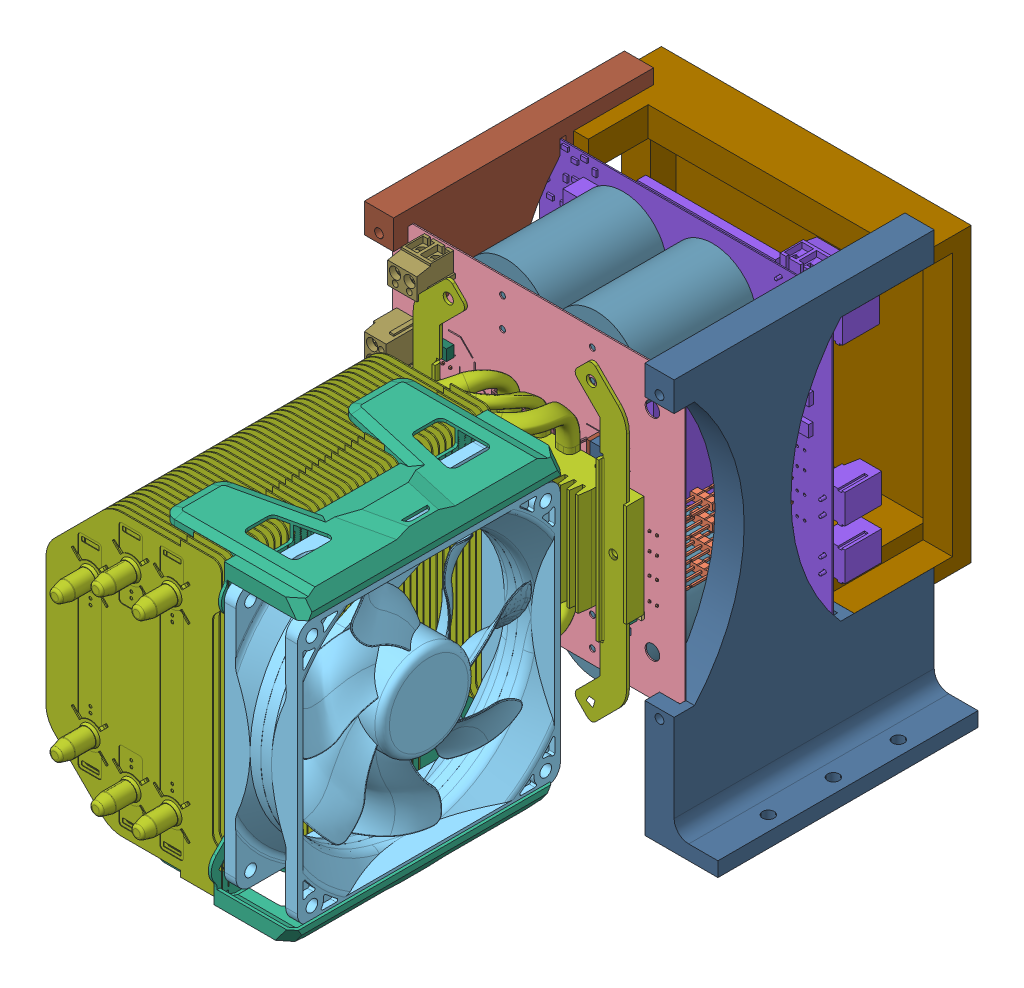
SolidWorks assembly conversor, configuration Default. Lengths in mm.
Overall size (196.64 140 240.72).
331 component instances, 30 part files, 12 mates.
Components (placement in the parent):
- inversor_rev2-1: inversor_rev2 [Default] at (-42.011 -49.0953 13.8297) size (100.07 109.25 61.05)
  - inversor_rev2.step-1: inversor_rev2.step [Default] at origin size (100.07 109.25 61.05)
    - R11.step-1: R11.step [Default] at origin size (1.4 2.15 0.65)
      - 1052595968.step-1: 1052595968.step [Default] at (72.136 29.972 0) size (1.4 2.15 0.65)
        - Extruded.step-1: Extruded.step [Default] at origin size (1.4 2.15 0.65)
    - R10.step-1: R10.step [Default] at origin size (1.4 2.15 0.65)
      - 1052595968.step-1: 1052595968.step [Default] at (74.93 29.972 0) size (1.4 2.15 0.65)
        - Extruded.step-1: Extruded.step [Default] at origin size (1.4 2.15 0.65)
    - P8.step-1: P8.step [Default] at origin size (7.72 2.67 47.1)
      - zl201-3_p2-54_l7-62_w2-54_h8-89.step-1: zl201-3_p2-54_l7-62_w2-54_h8-89.step [Default] at (83.5661 26.6699 -43.4013) x (1 0 0) z (0 -1 0) size (7.62 11.94 2.54)
      - zl201-3_p2-54_l7-62_w2-54_h8-89.step-2: zl201-3_p2-54_l7-62_w2-54_h8-89.step [Default] at (83.6675 26.7717 -20) x (1 0 0) z (0 -1 0) size (7.62 11.94 2.54)
      - zl201-3_p2-54_l7-62_w2-54_h8-89.step-3: zl201-3_p2-54_l7-62_w2-54_h8-89.step [Default] at (83.6675 26.7717 -2.4013) x (1 0 0) z (0 1 0) size (7.62 11.94 2.54)
      - zl201-3_p2-54_l7-62_w2-54_h8-89.step-4: zl201-3_p2-54_l7-62_w2-54_h8-89.step [Default] at (83.6675 26.7971 -31.9013) x (1 0 0) z (0 -1 0) size (7.62 11.94 2.54)
    - C19.step-1: C19.step [Default] at origin size (1.45 2.2 1.1)
      - 1052595832.step-1: 1052595832.step [Default] at (83.566 21.59 0) size (1.45 2.2 1.1)
        - Extruded-4.step-1: Extruded-4.step [Default] at origin size (1.45 2.2 1.1)
    - C18.step-1: C18.step [Default] at origin size (1.45 2.2 1.1)
      - 1052595832.step-1: 1052595832.step [Default] at (69.342 30.353 0) size (1.45 2.2 1.1)
        - Extruded-4.step-1: Extruded-4.step [Default] at origin size (1.45 2.2 1.1)
    - C11.step-1: C11.step [Default] at origin size (3.4 1.8 1.35)
      - 1052596240.step-1: 1052596240.step [Default] at (79.502 24.892 -1.7513) size (3.4 1.8 1.35)
        - Extruded-1.step-1: Extruded-1.step [Default] at origin size (3.4 1.8 1.35)
    - C10.step-1: C10.step [Default] at origin size (4.3 7.5 4)
      - 1052596648.step-1: 1052596648.step [Default] at (79.502 22.352 0) size (4.3 4.9 4)
        - Extruded-2.step-1: Extruded-2.step [Default] at origin size (4.3 4.9 4)
      - 1052596784.step-1: 1052596784.step [Default] at (79.502 19.252 0) size (4.3 1.3 4)
        - Extruded-3.step-1: Extruded-3.step [Default] at origin size (4.3 1.3 4)
      - 1052596784.step-2: 1052596784.step [Default] at (79.502 25.452 0) size (4.3 1.3 4)
        - Extruded-3.step-1: Extruded-3.step [Default] at origin size (4.3 1.3 4)
    - C22.step-1: C22.step [Default] at origin size (1.45 2.2 1.1)
      - 1052597056.step-1: 1052597056.step [Default] at (74.93 32.512 -1.7513) size (1.45 2.2 1.1)
        - Extruded-4.step-1: Extruded-4.step [Default] at origin size (1.45 2.2 1.1)
    - C21.step-1: C21.step [Default] at origin size (4.3 7.5 4)
      - 1052596648.step-1: 1052596648.step [Default] at (79.502 31.242 0) size (4.3 4.9 4)
        - Extruded-2.step-1: Extruded-2.step [Default] at origin size (4.3 4.9 4)
      - 1052596784.step-1: 1052596784.step [Default] at (79.502 28.142 0) size (4.3 1.3 4)
        - Extruded-3.step-1: Extruded-3.step [Default] at origin size (4.3 1.3 4)
      - 1052596784.step-2: 1052596784.step [Default] at (79.502 34.342 0) size (4.3 1.3 4)
        - Extruded-3.step-1: Extruded-3.step [Default] at origin size (4.3 1.3 4)
    - C20.step-1: C20.step [Default] at origin size (4.3 7.5 4)
      - 1052596648.step-1: 1052596648.step [Default] at (79.248 31.242 -4.4013) size (4.3 4.9 4)
        - Extruded-2.step-1: Extruded-2.step [Default] at origin size (4.3 4.9 4)
      - 1052596784.step-1: 1052596784.step [Default] at (79.248 28.142 -4.4013) size (4.3 1.3 4)
        - Extruded-3.step-1: Extruded-3.step [Default] at origin size (4.3 1.3 4)
      - 1052596784.step-2: 1052596784.step [Default] at (79.248 34.342 -4.4013) size (4.3 1.3 4)
        - Extruded-3.step-1: Extruded-3.step [Default] at origin size (4.3 1.3 4)
    - D3.step-1: D3.step [Default] at origin size (20 1.52 1.52)
      - do35_d1-5_l3.step-1: do35_d1-5_l3.step [Default] at (49.9079 33.2429 -1.4013) x (1 0 0) z (0 0 -1) size (20 1.52 1.52)
        - Open CASCADE STEP translator 6.8 1.12.1.1.step-1: Open CASCADE STEP translator 6.8 1.12.1.1.step [Default] at origin size (20 1.52 1.52)
        - Open CASCADE STEP translator 6.8 1.12.1.2.step-1: Open CASCADE STEP translator 6.8 1.12.1.2.step [Default] at origin
    - D2.step-1: D2.step [Default] at origin size (20 1.52 1.52)
      - do35_d1-5_l3.step-1: do35_d1-5_l3.step [Default] at (49.9619 38.0745 -1.4013) x (1 0 0) z (0 0 -1) size (20 1.52 1.52)
        - Open CASCADE STEP translator 6.8 1.12.1.1.step-1: Open CASCADE STEP translator 6.8 1.12.1.1.step [Default] at origin size (20 1.52 1.52)
        - Open CASCADE STEP translator 6.8 1.12.1.2.step-1: Open CASCADE STEP translator 6.8 1.12.1.2.step [Default] at origin
    - D1.step-1: D1.step [Default] at origin size (20 1.52 1.52)
      - do35_d1-5_l3.step-1: do35_d1-5_l3.step [Default] at (49.9959 42.6465 -1.4013) x (1 0 0) z (0 0 -1) size (20 1.52 1.52)
        - Open CASCADE STEP translator 6.8 1.12.1.1.step-1: Open CASCADE STEP translator 6.8 1.12.1.1.step [Default] at origin size (20 1.52 1.52)
        - Open CASCADE STEP translator 6.8 1.12.1.2.step-1: Open CASCADE STEP translator 6.8 1.12.1.2.step [Default] at origin
    - R13.step-1: R13.step [Default] at origin size (2.15 1.4 0.65)
      - 1052596104.step-1: 1052596104.step [Default] at (58.928 35.56 -1.0513) size (2.15 1.4 0.65)
        - Extruded-5.step-1: Extruded-5.step [Default] at origin size (2.15 1.4 0.65)
    - R15.step-1: R15.step [Default] at origin size (2.15 1.4 0.65)
      - 1052596104.step-1: 1052596104.step [Default] at (40.132 33.782 -1.0513) size (2.15 1.4 0.65)
        - Extruded-5.step-1: Extruded-5.step [Default] at origin size (2.15 1.4 0.65)
    - R14.step-1: R14.step [Default] at origin size (2.15 1.4 0.65)
      - 1052596104.step-1: 1052596104.step [Default] at (40.386 38.608 -1.0513) size (2.15 1.4 0.65)
        - Extruded-5.step-1: Extruded-5.step [Default] at origin size (2.15 1.4 0.65)
    - R12.step-1: R12.step [Default] at origin size (2.15 1.4 0.65)
      - 1052596104.step-1: 1052596104.step [Default] at (40.386 43.434 -1.0513) size (2.15 1.4 0.65)
        - Extruded-5.step-1: Extruded-5.step [Default] at origin size (2.15 1.4 0.65)
    - C26.step-1: C26.step [Default] at origin size (2.2 1.45 1.1)
      - 1052596920.step-1: 1052596920.step [Default] at (41.402 40.64 -1.5013) size (2.2 1.45 1.1)
        - Extruded-6.step-1: Extruded-6.step [Default] at origin size (2.2 1.45 1.1)
    - C25.step-1: C25.step [Default] at origin size (2.2 1.45 1.1)
      - 1052596920.step-1: 1052596920.step [Default] at (41.402 35.814 -1.5013) size (2.2 1.45 1.1)
        - Extruded-6.step-1: Extruded-6.step [Default] at origin size (2.2 1.45 1.1)
    - C24.step-1: C24.step [Default] at origin size (2.2 1.45 1.1)
      - 1052596920.step-1: 1052596920.step [Default] at (41.402 30.988 -1.5013) size (2.2 1.45 1.1)
        - Extruded-6.step-1: Extruded-6.step [Default] at origin size (2.2 1.45 1.1)
    - R17.step-1: R17.step [Default] at origin size (1.4 2.15 0.65)
      - 1052595968.step-1: 1052595968.step [Default] at (78.994 14.478 0) size (1.4 2.15 0.65)
        - Extruded.step-1: Extruded.step [Default] at origin size (1.4 2.15 0.65)
    - P1.step-1: P1.step [Default] at origin size (7.72 2.67 47.1)
      - zl201-3_p2-54_l7-62_w2-54_h8-89.step-1: zl201-3_p2-54_l7-62_w2-54_h8-89.step [Default] at (83.5661 34.2899 -43.4013) x (1 0 0) z (0 -1 0) size (7.62 11.94 2.54)
      - zl201-3_p2-54_l7-62_w2-54_h8-89.step-2: zl201-3_p2-54_l7-62_w2-54_h8-89.step [Default] at (83.6675 34.3917 -20) x (1 0 0) z (0 -1 0) size (7.62 11.94 2.54)
      - zl201-3_p2-54_l7-62_w2-54_h8-89.step-3: zl201-3_p2-54_l7-62_w2-54_h8-89.step [Default] at (83.6675 34.3917 -2.4013) x (1 0 0) z (0 1 0) size (7.62 11.94 2.54)
      - zl201-3_p2-54_l7-62_w2-54_h8-89.step-4: zl201-3_p2-54_l7-62_w2-54_h8-89.step [Default] at (83.6675 34.4171 -31.9013) x (1 0 0) z (0 -1 0) size (7.62 11.94 2.54)
    - C17.step-1: C17.step [Default] at origin size (2.2 1.45 1.1)
      - 1052596920.step-1: 1052596920.step [Default] at (75.946 47.498 -1.5013) size (2.2 1.45 1.1)
        - Extruded-6.step-1: Extruded-6.step [Default] at origin size (2.2 1.45 1.1)
    - C16.step-1: C16.step [Default] at origin size (2.2 1.45 1.1)
      - 1052596920.step-1: 1052596920.step [Default] at (75.946 41.402 -1.5013) size (2.2 1.45 1.1)
        - Extruded-6.step-1: Extruded-6.step [Default] at origin size (2.2 1.45 1.1)
    - C15.step-1: C15.step [Default] at origin size (2.2 1.45 1.1)
      - 1052596920.step-1: 1052596920.step [Default] at (75.946 45.466 -1.5013) size (2.2 1.45 1.1)
        - Extruded-6.step-1: Extruded-6.step [Default] at origin size (2.2 1.45 1.1)
    - C14.step-1: C14.step [Default] at origin size (2.2 1.45 1.1)
      - 1052596920.step-1: 1052596920.step [Default] at (75.946 39.37 -1.5013) size (2.2 1.45 1.1)
        - Extruded-6.step-1: Extruded-6.step [Default] at origin size (2.2 1.45 1.1)
    - C13.step-1: C13.step [Default] at origin size (2.2 1.45 1.1)
      - 1052596920.step-1: 1052596920.step [Default] at (75.946 43.434 -1.5013) size (2.2 1.45 1.1)
        - Extruded-6.step-1: Extruded-6.step [Default] at origin size (2.2 1.45 1.1)
    - C12.step-1: C12.step [Default] at origin size (2.2 1.45 1.1)
      - 1052596920.step-1: 1052596920.step [Default] at (75.946 37.338 -1.5013) size (2.2 1.45 1.1)
        - Extruded-6.step-1: Extruded-6.step [Default] at origin size (2.2 1.45 1.1)
    - P2.step-1: P2.step [Default] at origin size (7.72 2.67 47.1)
      - zl201-3_p2-54_l7-62_w2-54_h8-89.step-1: zl201-3_p2-54_l7-62_w2-54_h8-89.step [Default] at (83.5661 47.4979 -43.4013) x (1 0 0) z (0 -1 0) size (7.62 11.94 2.54)
      - zl201-3_p2-54_l7-62_w2-54_h8-89.step-2: zl201-3_p2-54_l7-62_w2-54_h8-89.step [Default] at (83.6675 47.5997 -20) x (1 0 0) z (0 -1 0) size (7.62 11.94 2.54)
      - zl201-3_p2-54_l7-62_w2-54_h8-89.step-3: zl201-3_p2-54_l7-62_w2-54_h8-89.step [Default] at (83.6675 47.5997 -2.4013) x (1 0 0) z (0 1 0) size (7.62 11.94 2.54)
      - zl201-3_p2-54_l7-62_w2-54_h8-89.step-4: zl201-3_p2-54_l7-62_w2-54_h8-89.step [Default] at (83.6675 47.6251 -31.9013) x (1 0 0) z (0 -1 0) size (7.62 11.94 2.54)
    - P3.step-1: P3.step [Default] at origin size (7.72 2.67 47.1)
      - zl201-3_p2-54_l7-62_w2-54_h8-89.step-1: zl201-3_p2-54_l7-62_w2-54_h8-89.step [Default] at (83.5661 41.5289 -43.4013) x (1 0 0) z (0 -1 0) size (7.62 11.94 2.54)
      - zl201-3_p2-54_l7-62_w2-54_h8-89.step-2: zl201-3_p2-54_l7-62_w2-54_h8-89.step [Default] at (83.6675 41.6307 -20) x (1 0 0) z (0 -1 0) size (7.62 11.94 2.54)
      - zl201-3_p2-54_l7-62_w2-54_h8-89.step-3: zl201-3_p2-54_l7-62_w2-54_h8-89.step [Default] at (83.6675 41.6307 -2.4013) x (1 0 0) z (0 1 0) size (7.62 11.94 2.54)
      - zl201-3_p2-54_l7-62_w2-54_h8-89.step-4: zl201-3_p2-54_l7-62_w2-54_h8-89.step [Default] at (83.6675 41.6561 -31.9013) x (1 0 0) z (0 -1 0) size (7.62 11.94 2.54)
    - R6.step-1: R6.step [Default] at origin size (2.15 1.4 0.65)
      - 1052596104.step-1: 1052596104.step [Default] at (75.946 37.338 0) size (2.15 1.4 0.65)
        - Extruded-5.step-1: Extruded-5.step [Default] at origin size (2.15 1.4 0.65)
    - R5.step-1: R5.step [Default] at origin size (2.15 1.4 0.65)
      - 1052596104.step-1: 1052596104.step [Default] at (75.946 39.37 0) size (2.15 1.4 0.65)
        - Extruded-5.step-1: Extruded-5.step [Default] at origin size (2.15 1.4 0.65)
    - R4.step-1: R4.step [Default] at origin size (2.15 1.4 0.65)
      - 1052596104.step-1: 1052596104.step [Default] at (75.946 41.402 0) size (2.15 1.4 0.65)
        - Extruded-5.step-1: Extruded-5.step [Default] at origin size (2.15 1.4 0.65)
    - R3.step-1: R3.step [Default] at origin size (2.15 1.4 0.65)
      - 1052596104.step-1: 1052596104.step [Default] at (75.946 43.434 0) size (2.15 1.4 0.65)
        - Extruded-5.step-1: Extruded-5.step [Default] at origin size (2.15 1.4 0.65)
    - R2.step-1: R2.step [Default] at origin size (2.15 1.4 0.65)
      - 1052596104.step-1: 1052596104.step [Default] at (75.946 45.466 0) size (2.15 1.4 0.65)
        - Extruded-5.step-1: Extruded-5.step [Default] at origin size (2.15 1.4 0.65)
    - R1.step-1: R1.step [Default] at origin size (2.15 1.4 0.65)
      - 1052596104.step-1: 1052596104.step [Default] at (75.946 47.498 0) size (2.15 1.4 0.65)
        - Extruded-5.step-1: Extruded-5.step [Default] at origin size (2.15 1.4 0.65)
    - C8.step-1: C8.step [Default] at origin size (7.5 4.3 4)
      - 1052596376.step-1: 1052596376.step [Default] at (75.211 51.816 0) size (4.9 4.3 4)
        - Extruded-7.step-1: Extruded-7.step [Default] at origin size (4.9 4.3 4)
      - 1052596512.step-1: 1052596512.step [Default] at (72.111 51.816 0) size (1.3 4.3 4)
        - Extruded-8.step-1: Extruded-8.step [Default] at origin size (1.3 4.3 4)
      - 1052596512.step-2: 1052596512.step [Default] at (78.311 51.816 0) size (1.3 4.3 4)
        - Extruded-8.step-1: Extruded-8.step [Default] at origin size (1.3 4.3 4)
    - C6.step-1: C6.step [Default] at origin size (7.5 4.3 4)
      - 1052596376.step-1: 1052596376.step [Default] at (71.855 58.928 0) size (4.9 4.3 4)
        - Extruded-7.step-1: Extruded-7.step [Default] at origin size (4.9 4.3 4)
      - 1052596512.step-1: 1052596512.step [Default] at (74.955 58.928 0) size (1.3 4.3 4)
        - Extruded-8.step-1: Extruded-8.step [Default] at origin size (1.3 4.3 4)
      - 1052596512.step-2: 1052596512.step [Default] at (68.755 58.928 0) size (1.3 4.3 4)
        - Extruded-8.step-1: Extruded-8.step [Default] at origin size (1.3 4.3 4)
    - C4.step-1: C4.step [Default] at origin size (7.5 4.3 4)
      - 1052596376.step-1: 1052596376.step [Default] at (72.136 65.786 0) size (4.9 4.3 4)
        - Extruded-7.step-1: Extruded-7.step [Default] at origin size (4.9 4.3 4)
      - 1052596512.step-1: 1052596512.step [Default] at (75.236 65.786 0) size (1.3 4.3 4)
        - Extruded-8.step-1: Extruded-8.step [Default] at origin size (1.3 4.3 4)
      - 1052596512.step-2: 1052596512.step [Default] at (69.036 65.786 0) size (1.3 4.3 4)
        - Extruded-8.step-1: Extruded-8.step [Default] at origin size (1.3 4.3 4)
    - -VDC1.step-1: -VDC1.step [Default] at origin size (10.6 9 17)
      - SCREW_TERMINAL_BLOCK_5MM.step-1: SCREW_TERMINAL_BLOCK_5MM.step [Default] at (20.1591 6.4347 2) x (-1 0 0) z (0 1 0) size (10.6 17 9)
    - +VDC1.step-1: +VDC1.step [Default] at origin size (10.6 9 17)
      - SCREW_TERMINAL_BLOCK_5MM.step-1: SCREW_TERMINAL_BLOCK_5MM.step [Default] at (10.9959 90.0853 2) x (1 0 0) z (0 -1 0) size (10.6 17 9)
    - P7.step-1: P7.step [Default] at origin size (7.72 2.67 47.1)
      - zl201-3_p2-54_l7-62_w2-54_h8-89.step-1: zl201-3_p2-54_l7-62_w2-54_h8-89.step [Default] at (18.0339 26.1621 -43.4013) x (-1 0 0) z (0 1 0) size (7.62 11.94 2.54)
      - zl201-3_p2-54_l7-62_w2-54_h8-89.step-2: zl201-3_p2-54_l7-62_w2-54_h8-89.step [Default] at (17.9325 26.0603 -20) x (-1 0 0) z (0 1 0) size (7.62 11.94 2.54)
      - zl201-3_p2-54_l7-62_w2-54_h8-89.step-3: zl201-3_p2-54_l7-62_w2-54_h8-89.step [Default] at (17.9325 26.0603 -2.4013) x (-1 0 0) z (0 -1 0) size (7.62 11.94 2.54)
      - zl201-3_p2-54_l7-62_w2-54_h8-89.step-4: zl201-3_p2-54_l7-62_w2-54_h8-89.step [Default] at (17.9325 26.0349 -31.9013) x (-1 0 0) z (0 1 0) size (7.62 11.94 2.54)
    - P6.step-1: P6.step [Default] at origin size (7.72 2.67 47.1)
      - zl201-3_p2-54_l7-62_w2-54_h8-89.step-1: zl201-3_p2-54_l7-62_w2-54_h8-89.step [Default] at (18.0339 35.8141 -43.4013) x (-1 0 0) z (0 1 0) size (7.62 11.94 2.54)
      - zl201-3_p2-54_l7-62_w2-54_h8-89.step-2: zl201-3_p2-54_l7-62_w2-54_h8-89.step [Default] at (17.9325 35.7123 -20) x (-1 0 0) z (0 1 0) size (7.62 11.94 2.54)
      - zl201-3_p2-54_l7-62_w2-54_h8-89.step-3: zl201-3_p2-54_l7-62_w2-54_h8-89.step [Default] at (17.9325 35.7123 -2.4013) x (-1 0 0) z (0 -1 0) size (7.62 11.94 2.54)
      - zl201-3_p2-54_l7-62_w2-54_h8-89.step-4: zl201-3_p2-54_l7-62_w2-54_h8-89.step [Default] at (17.9325 35.6869 -31.9013) x (-1 0 0) z (0 1 0) size (7.62 11.94 2.54)
    - P5.step-1: P5.step [Default] at origin size (7.72 2.67 47.1)
      - zl201-3_p2-54_l7-62_w2-54_h8-89.step-1: zl201-3_p2-54_l7-62_w2-54_h8-89.step [Default] at (18.0339 50.0381 -43.4013) x (-1 0 0) z (0 1 0) size (7.62 11.94 2.54)
      - zl201-3_p2-54_l7-62_w2-54_h8-89.step-2: zl201-3_p2-54_l7-62_w2-54_h8-89.step [Default] at (17.9325 49.9363 -20) x (-1 0 0) z (0 1 0) size (7.62 11.94 2.54)
      - zl201-3_p2-54_l7-62_w2-54_h8-89.step-3: zl201-3_p2-54_l7-62_w2-54_h8-89.step [Default] at (17.9325 49.9363 -2.4013) x (-1 0 0) z (0 -1 0) size (7.62 11.94 2.54)
      - zl201-3_p2-54_l7-62_w2-54_h8-89.step-4: zl201-3_p2-54_l7-62_w2-54_h8-89.step [Default] at (17.9325 49.9109 -31.9013) x (-1 0 0) z (0 1 0) size (7.62 11.94 2.54)
    - P4.step-1: P4.step [Default] at origin size (7.72 2.67 47.1)
      - zl201-3_p2-54_l7-62_w2-54_h8-89.step-1: zl201-3_p2-54_l7-62_w2-54_h8-89.step [Default] at (18.0339 61.9761 -43.4013) x (-1 0 0) z (0 1 0) size (7.62 11.94 2.54)
      - zl201-3_p2-54_l7-62_w2-54_h8-89.step-2: zl201-3_p2-54_l7-62_w2-54_h8-89.step [Default] at (17.9325 61.8743 -20) x (-1 0 0) z (0 1 0) size (7.62 11.94 2.54)
      - zl201-3_p2-54_l7-62_w2-54_h8-89.step-3: zl201-3_p2-54_l7-62_w2-54_h8-89.step [Default] at (17.9325 61.8743 -2.4013) x (-1 0 0) z (0 -1 0) size (7.62 11.94 2.54)
      - zl201-3_p2-54_l7-62_w2-54_h8-89.step-4: zl201-3_p2-54_l7-62_w2-54_h8-89.step [Default] at (17.9325 61.8489 -31.9013) x (-1 0 0) z (0 1 0) size (7.62 11.94 2.54)
    - W1.step-1: W1.step [Default] at origin size (9 10.6 17)
      - SCREW_TERMINAL_BLOCK_5MM.step-1: SCREW_TERMINAL_BLOCK_5MM.step [Default] at (10.4987 39.4909 2) x (0 1 0) z (1 0 0) size (10.6 17 9)
    - V1.step-1: V1.step [Default] at origin size (9 10.6 17)
      - SCREW_TERMINAL_BLOCK_5MM.step-1: SCREW_TERMINAL_BLOCK_5MM.step [Default] at (10.4987 50.9209 2) x (0 1 0) z (1 0 0) size (10.6 17 9)
    - U1.step-1: U1.step [Default] at origin size (9 10.6 17)
      - SCREW_TERMINAL_BLOCK_5MM.step-1: SCREW_TERMINAL_BLOCK_5MM.step [Default] at (10.4987 62.3509 2) x (0 1 0) z (1 0 0) size (10.6 17 9)
    - C3.step-1: C3.step [Default] at origin size (3.4 1.8 1.35)
      - 1052596240.step-1: 1052596240.step [Default] at (16.51 52.578 -1.7513) size (3.4 1.8 1.35)
        - Extruded-1.step-1: Extruded-1.step [Default] at origin size (3.4 1.8 1.35)
    - C2.step-1: C2.step [Default] at origin size (3.4 1.8 1.35)
      - 1052596240.step-1: 1052596240.step [Default] at (16.637 64.516 -1.7513) size (3.4 1.8 1.35)
        - Extruded-1.step-1: Extruded-1.step [Default] at origin size (3.4 1.8 1.35)
    - C1.step-1: C1.step [Default] at origin size (3.4 1.8 1.35)
      - 1052596240.step-1: 1052596240.step [Default] at (16.51 38.354 -1.7513) size (3.4 1.8 1.35)
        - Extruded-1.step-1: Extruded-1.step [Default] at origin size (3.4 1.8 1.35)
    - U2.step-1: U2.step [Default] at origin size (29.83 36.3 7.7)
      - User_Library-Cipos-mini-PCB.step-1: User_Library-Cipos-mini-PCB.step [Default] at (38.058 67.0707 2.5987) x (0 1 0) z (1 0 0) size (36.3 7.7 29.83)
    - C7.step-1: C7.step [Default] at origin size (7.5 4.3 4)
      - 1052596376.step-1: 1052596376.step [Default] at (72.136 58.928 -4.4013) size (4.9 4.3 4)
        - Extruded-7.step-1: Extruded-7.step [Default] at origin size (4.9 4.3 4)
      - 1052596512.step-1: 1052596512.step [Default] at (75.236 58.928 -4.4013) size (1.3 4.3 4)
        - Extruded-8.step-1: Extruded-8.step [Default] at origin size (1.3 4.3 4)
      - 1052596512.step-2: 1052596512.step [Default] at (69.036 58.928 -4.4013) size (1.3 4.3 4)
        - Extruded-8.step-1: Extruded-8.step [Default] at origin size (1.3 4.3 4)
    - C5.step-1: C5.step [Default] at origin size (7.5 4.3 4)
      - 1052596376.step-1: 1052596376.step [Default] at (71.882 65.786 -4.4013) size (4.9 4.3 4)
        - Extruded-7.step-1: Extruded-7.step [Default] at origin size (4.9 4.3 4)
      - 1052596512.step-1: 1052596512.step [Default] at (74.982 65.786 -4.4013) size (1.3 4.3 4)
        - Extruded-8.step-1: Extruded-8.step [Default] at origin size (1.3 4.3 4)
      - 1052596512.step-2: 1052596512.step [Default] at (68.782 65.786 -4.4013) size (1.3 4.3 4)
        - Extruded-8.step-1: Extruded-8.step [Default] at origin size (1.3 4.3 4)
    - C9.step-1: C9.step [Default] at origin size (7.5 4.3 4)
      - 1052596376.step-1: 1052596376.step [Default] at (75.184 51.562 -4.4013) size (4.9 4.3 4)
        - Extruded-7.step-1: Extruded-7.step [Default] at origin size (4.9 4.3 4)
      - 1052596512.step-1: 1052596512.step [Default] at (72.084 51.562 -4.4013) size (1.3 4.3 4)
        - Extruded-8.step-1: Extruded-8.step [Default] at origin size (1.3 4.3 4)
      - 1052596512.step-2: 1052596512.step [Default] at (78.284 51.562 -4.4013) size (1.3 4.3 4)
        - Extruded-8.step-1: Extruded-8.step [Default] at origin size (1.3 4.3 4)
    - C_bus2.step-1: C_bus2.step [Default] at origin size (30 30 40)
      - 1152675632.step-1: 1152675632.step [Default] at (66.2941 87.0713 -1.4013) x (0 1 0) z (0 0 -1) size (30 30 40)
        - Cylinder.step-1: Cylinder.step [Default] at origin size (30 30 40)
    - C_bus1.step-1: C_bus1.step [Default] at origin size (30 30 40)
      - 1152675632.step-1: 1152675632.step [Default] at (35.5601 87.1221 -1.4013) x (0 1 0) z (0 0 -1) size (30 30 40)
        - Cylinder.step-1: Cylinder.step [Default] at origin size (30 30 40)
    - C_bus4.step-1: C_bus4.step [Default] at origin size (30 30 40)
      - 1152675632.step-1: 1152675632.step [Default] at (35.5601 7.8741 -1.4013) x (0 1 0) z (0 0 -1) size (30 30 40)
        - Cylinder.step-1: Cylinder.step [Default] at origin size (30 30 40)
    - C_bus3.step-1: C_bus3.step [Default] at origin size (30 30 40)
      - 1152675632.step-1: 1152675632.step [Default] at (66.2941 7.8741 -1.4013) x (0 1 0) z (0 0 -1) size (30 30 40)
        - Cylinder.step-1: Cylinder.step [Default] at origin size (30 30 40)
    - CC1.step-1: CC1.step [Default] at origin size (5 3.8 2.55)
      - 1052597192.step-1: 1052597192.step [Default] at (16.6678 67.3928 0.1) size (5 3.8 2.55)
        - Extruded-9.step-1: Extruded-9.step [Default] at origin size (5 3.8 2.55)
    - CC2.step-1: CC2.step [Default] at origin size (5 3.8 2.55)
      - 1052597192.step-1: 1052597192.step [Default] at (16.6678 54.9722 0.1) size (5 3.8 2.55)
        - Extruded-9.step-1: Extruded-9.step [Default] at origin size (5 3.8 2.55)
    - CC3.step-1: CC3.step [Default] at origin size (5 3.8 2.55)
      - 1052597192.step-1: 1052597192.step [Default] at (16.9726 40.9768 0.1) size (5 3.8 2.55)
        - Extruded-9.step-1: Extruded-9.step [Default] at origin size (5 3.8 2.55)
    - C27.step-1: C27.step [Default] at origin size (2.2 1.45 1.1)
      - 1052596920.step-1: 1052596920.step [Default] at (4.572 25.4 -1.5013) size (2.2 1.45 1.1)
        - Extruded-6.step-1: Extruded-6.step [Default] at origin size (2.2 1.45 1.1)
    - C28.step-1: C28.step [Default] at origin size (2.2 1.45 1.1)
      - 1052596920.step-1: 1052596920.step [Default] at (4.572 27.432 -1.5013) size (2.2 1.45 1.1)
        - Extruded-6.step-1: Extruded-6.step [Default] at origin size (2.2 1.45 1.1)
    - C29.step-1: C29.step [Default] at origin size (1.45 2.2 1.1)
      - 1052595832.step-1: 1052595832.step [Default] at (1.778 31.369 -1.5013) size (1.45 2.2 1.1)
        - Extruded-4.step-1: Extruded-4.step [Default] at origin size (1.45 2.2 1.1)
    - C30.step-1: C30.step [Default] at origin size (2.2 1.45 1.1)
      - 1052596920.step-1: 1052596920.step [Default] at (13.716 28.448 0) size (2.2 1.45 1.1)
        - Extruded-6.step-1: Extruded-6.step [Default] at origin size (2.2 1.45 1.1)
    - C31.step-1: C31.step [Default] at origin size (1.45 2.2 1.1)
      - 1052595832.step-1: 1052595832.step [Default] at (18.542 30.734 -1.5013) size (1.45 2.2 1.1)
        - Extruded-4.step-1: Extruded-4.step [Default] at origin size (1.45 2.2 1.1)
    - R7.step-1: R7.step [Default] at origin size (6.65 3.45 0.9)
      - 1152666032.step-1: 1152666032.step [Default] at (28.5496 41.529 0) x (-1 0 0) z (0 0 1) size (6.65 3.45 0.9)
        - Terminal.step-1: Terminal.step [Default] at (-3.325 -1.725 0) size (0.6 3.45 0.9)
          - Open_CASCADE_STEP_translator_6.8_1.2.1.step-1: Open_CASCADE_STEP_translator_6.8_1.2.1.step [Default] at origin size (0.6 3.45 0.9)
        - Terminal.step-2: Terminal.step [Default] at (3.325 1.725 0) x (-1 0 0) z (0 0 1) size (0.6 3.45 0.9)
          - Open_CASCADE_STEP_translator_6.8_1.2.1.step-1: Open_CASCADE_STEP_translator_6.8_1.2.1.step [Default] at origin size (0.6 3.45 0.9)
        - Mid_Body.step-1: Mid_Body.step [Default] at (-3.325 -1.725 0) size (6.47 3.45 0.72)
        - Mark.step-1: Mark.step [Default] at (-2.725 -1.725 0.81) size (5.45 3.45 0.09)
    - R8.step-1: R8.step [Default] at origin size (6.65 3.45 0.9)
      - 1152666032.step-1: 1152666032.step [Default] at (28.5496 36.8808 -0.4013) x (-1 0 0) z (0 0 -1) size (6.65 3.45 0.9)
        - Terminal.step-1: Terminal.step [Default] at (-3.325 -1.725 0) size (0.6 3.45 0.9)
          - Open_CASCADE_STEP_translator_6.8_1.2.1.step-1: Open_CASCADE_STEP_translator_6.8_1.2.1.step [Default] at origin size (0.6 3.45 0.9)
        - Terminal.step-2: Terminal.step [Default] at (3.325 1.725 0) x (-1 0 0) z (0 0 1) size (0.6 3.45 0.9)
          - Open_CASCADE_STEP_translator_6.8_1.2.1.step-1: Open_CASCADE_STEP_translator_6.8_1.2.1.step [Default] at origin size (0.6 3.45 0.9)
        - Mid_Body.step-1: Mid_Body.step [Default] at (-3.325 -1.725 0) size (6.47 3.45 0.72)
        - Mark.step-1: Mark.step [Default] at (-2.725 -1.725 0.81) size (5.45 3.45 0.09)
    - R9.step-1: R9.step [Default] at origin size (6.65 3.45 0.9)
      - 1152666032.step-1: 1152666032.step [Default] at (28.5496 32.3342 0) x (-1 0 0) z (0 0 1) size (6.65 3.45 0.9)
        - Terminal.step-1: Terminal.step [Default] at (-3.325 -1.725 0) size (0.6 3.45 0.9)
          - Open_CASCADE_STEP_translator_6.8_1.2.1.step-1: Open_CASCADE_STEP_translator_6.8_1.2.1.step [Default] at origin size (0.6 3.45 0.9)
        - Terminal.step-2: Terminal.step [Default] at (3.325 1.725 0) x (-1 0 0) z (0 0 1) size (0.6 3.45 0.9)
          - Open_CASCADE_STEP_translator_6.8_1.2.1.step-1: Open_CASCADE_STEP_translator_6.8_1.2.1.step [Default] at origin size (0.6 3.45 0.9)
        - Mid_Body.step-1: Mid_Body.step [Default] at (-3.325 -1.725 0) size (6.47 3.45 0.72)
        - Mark.step-1: Mark.step [Default] at (-2.725 -1.725 0.81) size (5.45 3.45 0.09)
    - R22.step-1: R22.step [Default] at origin size (1.4 2.15 0.65)
      - 1052595968.step-1: 1052595968.step [Default] at (12.7 31.48 0) size (1.4 2.15 0.65)
        - Extruded.step-1: Extruded.step [Default] at origin size (1.4 2.15 0.65)
    - R23.step-1: R23.step [Default] at origin size (1.4 2.15 0.65)
      - 1052595968.step-1: 1052595968.step [Default] at (-0.508 31.369 -1.0513) size (1.4 2.15 0.65)
        - Extruded.step-1: Extruded.step [Default] at origin size (1.4 2.15 0.65)
    - R19.step-1: R19.step [Default] at origin size (1.4 2.15 0.65)
      - 1052595968.step-1: 1052595968.step [Default] at (-0.508 77.268 -1.0513) size (1.4 2.15 0.65)
        - Extruded.step-1: Extruded.step [Default] at origin size (1.4 2.15 0.65)
    - R20.step-1: R20.step [Default] at origin size (1.4 2.15 0.65)
      - 1052595968.step-1: 1052595968.step [Default] at (-0.508 72.95 -1.0513) size (1.4 2.15 0.65)
        - Extruded.step-1: Extruded.step [Default] at origin size (1.4 2.15 0.65)
    - R21.step-1: R21.step [Default] at origin size (1.4 2.15 0.65)
      - 1052595968.step-1: 1052595968.step [Default] at (-0.508 68.632 -1.0513) size (1.4 2.15 0.65)
        - Extruded.step-1: Extruded.step [Default] at origin size (1.4 2.15 0.65)
    - R25.step-1: R25.step [Default] at origin size (1.4 2.15 0.65)
      - 1052595968.step-1: 1052595968.step [Default] at (-0.4698 18.2106 -1.0513) size (1.4 2.15 0.65)
        - Extruded.step-1: Extruded.step [Default] at origin size (1.4 2.15 0.65)
    - R26.step-1: R26.step [Default] at origin size (1.4 2.15 0.65)
      - 1052595968.step-1: 1052595968.step [Default] at (-0.4698 22.5286 -1.0513) size (1.4 2.15 0.65)
        - Extruded.step-1: Extruded.step [Default] at origin size (1.4 2.15 0.65)
    - R27.step-1: R27.step [Default] at origin size (1.4 2.15 0.65)
      - 1052595968.step-1: 1052595968.step [Default] at (-0.4698 26.8466 -1.0513) size (1.4 2.15 0.65)
        - Extruded.step-1: Extruded.step [Default] at origin size (1.4 2.15 0.65)
    - U3.step-1: U3.step [Default] at origin size (15.89 5.82 7)
      - 1052597328.step-1: 1052597328.step [Default] at (8.8002 21.2217 -8.4013) size (15.89 5.82 7)
        - Extruded-10.step-1: Extruded-10.step [Default] at origin size (15.89 5.82 7)
    - U4.step-1: U4.step [Default] at origin size (7.52 5.21 2.8)
      - 1052597736.step-1: 1052597736.step [Default] at (9.525 31.3817 -3.4013) size (7.52 5.21 2.8)
        - Extruded-11.step-1: Extruded-11.step [Default] at origin size (7.52 5.21 2.8)
    - C_bus5.step-1: C_bus5.step [Default] at origin size (7.9 24.84 2)
      - 1052597464.step-1: 1052597464.step [Default] at (22.3139 52.7051 -3.4013) size (7.9 24.84 2)
        - Extruded-12.step-1: Extruded-12.step [Default] at origin size (7.9 24.84 2)
    - R16.step-1: R16.step [Default] at origin size (2.15 1.4 0.65)
      - 1052596104.step-1: 1052596104.step [Default] at (59.436 30.226 -1.0513) size (2.15 1.4 0.65)
        - Extruded-5.step-1: Extruded-5.step [Default] at origin size (2.15 1.4 0.65)
    - C23.step-1: C23.step [Default] at origin size (2.2 1.45 1.1)
      - 1052596920.step-1: 1052596920.step [Default] at (66.548 33.782 -1.5013) size (2.2 1.45 1.1)
        - Extruded-6.step-1: Extruded-6.step [Default] at origin size (2.2 1.45 1.1)
    - R18.step-1: R18.step [Default] at origin size (1.4 2.15 0.65)
      - 1052595968.step-1: 1052595968.step [Default] at (-0.508 81.534 -1.0513) size (1.4 2.15 0.65)
        - Extruded.step-1: Extruded.step [Default] at origin size (1.4 2.15 0.65)
    - R24.step-1: R24.step [Default] at origin size (2.15 1.4 0.65)
      - 1052596104.step-1: 1052596104.step [Default] at (0.508 15.113 -1.0513) size (2.15 1.4 0.65)
        - Extruded-5.step-1: Extruded-5.step [Default] at origin size (2.15 1.4 0.65)
    - Board.step-1: Board.step [Default] at origin size (100.07 99.8 0.41)
- heatsink-1: heatsink [Default] at (-0.3777 43.1754 102.4783) x (0 -1 0) z (0 0 1) size (108.44 180.01 139.76)
  - 7030025_PART_FAN STANDARD 90_MODEL.igs-1: 7030025_PART_FAN STANDARD 90_MODEL.igs [Default] at (0 45 -45) x (1 0 0) z (0 -1 0) size (93.98 180.01 25.07)
  - 7030026_PART_HEATSINK ADAPTOR 90_MODEL.igs-1: 7030026_PART_HEATSINK ADAPTOR 90_MODEL.igs [Default] at (95 58.5 47.4641) x (0 0 -1) z (-1 0 0) size (106.39 52.6 26.58)
  - 7030026_PART_HEATSINK ADAPTOR 90_MODEL.igs-2: 7030026_PART_HEATSINK ADAPTOR 90_MODEL.igs [Default] at (-7 58.5 -46) x (0 0 1) z (1 0 0) size (106.39 52.6 26.58)
  - 7030027_PART_CPU HEATSINK TOWER_MODEL.igs-1: 7030027_PART_CPU HEATSINK TOWER_MODEL.igs [Default] at (94 31.5 -47.65) x (-1 0 0) z (0 0 1) size (108.44 80.01 139.76)
- controlo_rev2-1: controlo_rev2 [Default] at (-42.011 -49.0953 -36.5818) size (103.49 101.24 40.41)
- suporte_topo-1: suporte_topo [Default] at (5.989 -1.0953 -41.2332) x (-1 0 0) z (0 -1 0) size (106 40 100)
- suporte_conversor_frente-3: suporte_conversor_frente [Default] at (48.989 -1.0953 -11.5818) x (0 1 0) z (1 0 0) size (140 89 25)
- suporte_conversor_trás-1: suporte_conversor_trás [Default] at (-37.011 -1.0953 -11.5818) x (0 -1 0) z (-1 0 0) size (140 89 25)
Mates (geometry in assembly coordinates):
- Tangent1: tangent: plane of inversor_rev2-1/inversor_rev2.step-1/U2.step-1/User_Library-Cipos-mini-PCB.step-1 through (4.347 16.7254 19.8283) normal (0 0 1); face of heatsink-1/7030027_PART_CPU HEATSINK TOWER_MODEL.igs-1
- Tangent2: tangent: plane of inversor_rev2-1/inversor_rev2.step-1/U2.step-1/User_Library-Cipos-mini-PCB.step-1 through (-3.953 -18.3246 19.8283) normal (0 -1 0); face of heatsink-1/7030027_PART_CPU HEATSINK TOWER_MODEL.igs-1
- Lock1: lock: unknown of inversor_rev2-1/inversor_rev2.step-1/Board.step-1; unknown of heatsink-1/7030027_PART_CPU HEATSINK TOWER_MODEL.igs-1
- Concentric1: concentric: cylinder of inversor_rev2-1/inversor_rev2.step-1/Board.step-1 through (-42.011 46.9047 13.4182) axis (0 0 -1) radius 1.5; cylinder of controlo_rev2-1 through (-42.011 46.9047 -36.9933) axis (0 0 -1) radius 1.5
- Concentric2: concentric: cylinder of inversor_rev2-1/inversor_rev2.step-1/Board.step-1 through (-42.011 -49.0953 13.4182) axis (0 0 -1) radius 1.5; cylinder of controlo_rev2-1 through (-42.011 -49.0953 -36.9933) axis (0 0 -1) radius 1.5
- Distance1: distance = 50 mm: plane of inversor_rev2-1/inversor_rev2.step-1/Board.step-1 through (-44.011 -51.0003 13.4182) normal (0 0 -1); plane of controlo_rev2-1 through (-44.011 -51.0003 -36.5818) normal (0 0 1)
- Coincident9: coincident: plane of inversor_rev2-1/inversor_rev2.step-1/Board.step-1 through (-44.011 -51.0003 13.4182) normal (0 0 -1); plane of suporte_conversor_frente-3 through (58.989 -1.0953 13.4182) normal (0 0 1)
- Concentric5: concentric: circle of inversor_rev2-1/inversor_rev2.step-1/Board.step-1; circle of suporte_conversor_frente-3
- Concentric6: concentric: cylinder of inversor_rev2-1/inversor_rev2.step-1/Board.step-1 through (53.989 46.9047 13.4182) axis (0 0 -1) radius 1.5; cylinder of suporte_conversor_frente-3 through (53.989 46.9047 24.6608) axis (0 0 -1) radius 1.5
- Coincident11: coincident: plane of inversor_rev2-1/inversor_rev2.step-1/Board.step-1 through (-44.011 -51.0003 13.4182) normal (0 0 -1); plane of suporte_conversor_trás-1 through (-47.011 -1.0953 13.4182) normal (0 0 1)
- Coincident12: coincident: cylinder of inversor_rev2-1/inversor_rev2.step-1/Board.step-1 through (-42.011 46.9047 13.4182) axis (0 0 -1) radius 1.5; circle of suporte_conversor_trás-1
- Coincident13: coincident: circle of inversor_rev2-1/inversor_rev2.step-1/Board.step-1; cylinder of suporte_conversor_trás-1 through (-42.011 -49.0953 24.6608) axis (0 0 -1) radius 1.5
